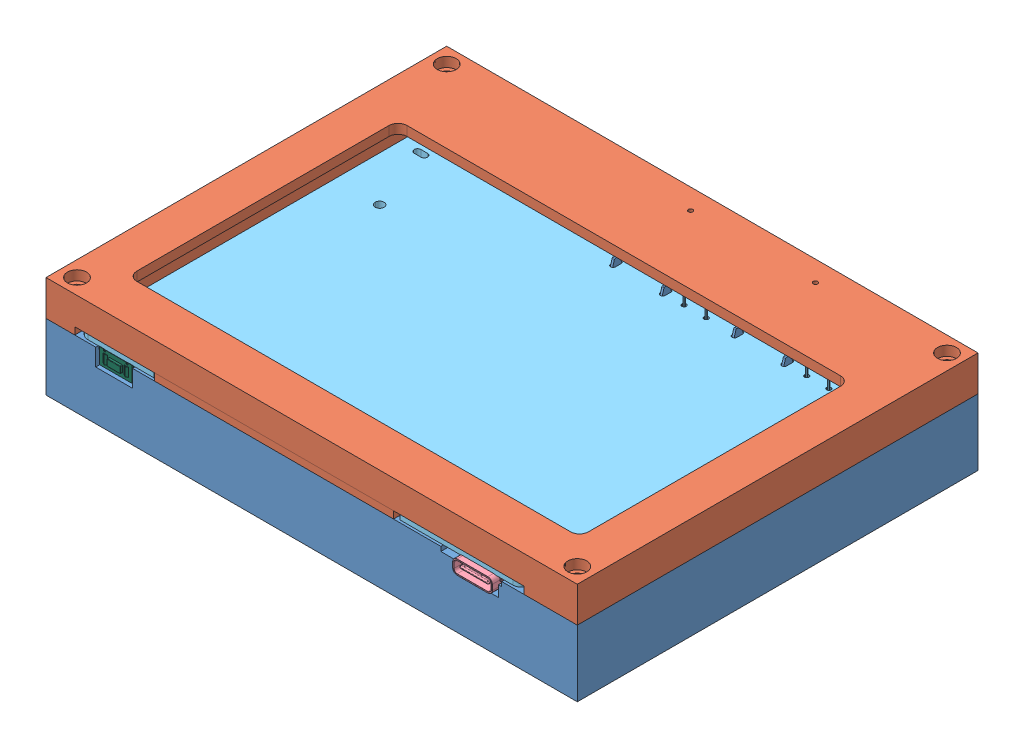
SolidWorks assembly 装配体2, configuration 默认. Lengths in mm.
Overall size (120 23 100.01).
848 component instances, 41 part files, 5 mates.
Components (placement in the parent):
- 底板-1: 底板 [默认] at (-10.6932 -23.0305 0) size (120 15 90.5)
- 面板-1: 面板 [默认] at (-10.6932 -0.0305 0) x (-1 0 0) z (0 0 1) size (120 8 90.5)
- 3D_board_2024-11-06-1: 3D_board_2024-11-06 [默认] at (-63.7814 -6.4105 44.7375) x (1 0 0) z (0 -1 0) size (99.97 100.01 16.2)
  - 3D_board_2024-11-06.step-1: 3D_board_2024-11-06.step [默认] at origin size (99.97 100.01 16.2)
    - iqks-X1.step-1: iqks-X1.step [默认] at (20.955 -9.525 1.5862) x (-1 0 0) z (0 0 1) size (3.2 2.5 0.81)
      - OSC-SMD_4P-L3.2-W2.5-BL.step-1: OSC-SMD_4P-L3.2-W2.5-BL.step [默认] at origin size (3.2 2.5 0.81)
        - SOLID.step-1: SOLID.step [默认] at origin size (3.2 2.5 0.81)
    - iqks-X2.step-1: iqks-X2.step [默认] at (48.2601 -24.765 1.5862) x (-1 0 0) z (0 0 1) size (7 5 1.32)
      - OSC-SMD_4P-L7.0-W5.0-BL.step-1: OSC-SMD_4P-L7.0-W5.0-BL.step [默认] at origin size (7 5 1.32)
        - COMPOUND.step-1: COMPOUND.step [默认] at origin size (7 5 1.32)
    - iqks-U22.step-1: iqks-U22.step [默认] at (45.7201 -54.6101 1.5862) x (-1 0 0) z (0 0 1) size (5.89 7.71 1.66)
      - SSOP-28_L10.2-W5.3-P0.65-LS7.8-BL.step-1: SSOP-28_L10.2-W5.3-P0.65-LS7.8-BL.step [默认] at origin size (5.89 7.71 1.66)
        - SOLID-0.step-1: SOLID-0.step [默认] at origin size (5.89 7.71 1.66)
    - iqks-RN4.step-1: iqks-RN4.step [默认] at (33.0201 -35.5601 1.5862) x (-1 0 0) z (0 0 1) size (3.2 1.6 0.5)
      - RES-ARRAY-SMD_0603-8P-L3.2-W1.6-BL.step-1: RES-ARRAY-SMD_0603-8P-L3.2-W1.6-BL.step [默认] at origin size (3.2 1.6 0.5)
        - COMPOUND-1.step-1: COMPOUND-1.step [默认] at origin size (3.2 1.6 0.5)
    - iqks-RN3.step-1: iqks-RN3.step [默认] at (29.2101 -35.5601 1.5862) x (-1 0 0) z (0 0 1) size (3.2 1.6 0.5)
      - RES-ARRAY-SMD_0603-8P-L3.2-W1.6-BL.step-1: RES-ARRAY-SMD_0603-8P-L3.2-W1.6-BL.step [默认] at origin size (3.2 1.6 0.5)
        - COMPOUND-1.step-1: COMPOUND-1.step [默认] at origin size (3.2 1.6 0.5)
    - iqks-RN2.step-1: iqks-RN2.step [默认] at (25.4001 -35.5601 1.5862) x (-1 0 0) z (0 0 1) size (3.2 1.6 0.5)
      - RES-ARRAY-SMD_0603-8P-L3.2-W1.6-BL.step-1: RES-ARRAY-SMD_0603-8P-L3.2-W1.6-BL.step [默认] at origin size (3.2 1.6 0.5)
        - COMPOUND-1.step-1: COMPOUND-1.step [默认] at origin size (3.2 1.6 0.5)
    - iqks-RN1.step-1: iqks-RN1.step [默认] at (21.59 -35.5601 1.5862) x (-1 0 0) z (0 0 1) size (3.2 1.6 0.5)
      - RES-ARRAY-SMD_0603-8P-L3.2-W1.6-BL.step-1: RES-ARRAY-SMD_0603-8P-L3.2-W1.6-BL.step [默认] at origin size (3.2 1.6 0.5)
        - COMPOUND-1.step-1: COMPOUND-1.step [默认] at origin size (3.2 1.6 0.5)
    - iqks-RN5.step-1: iqks-RN5.step [默认] at (36.8301 -35.5601 1.5862) x (-1 0 0) z (0 0 1) size (3.2 1.6 0.5)
      - RES-ARRAY-SMD_0603-8P-L3.2-W1.6-BL.step-1: RES-ARRAY-SMD_0603-8P-L3.2-W1.6-BL.step [默认] at origin size (3.2 1.6 0.5)
        - COMPOUND-1.step-1: COMPOUND-1.step [默认] at origin size (3.2 1.6 0.5)
    - iqks-R53.step-1: iqks-R53.step [默认] at (90.8052 -10.16 1.5862) x (0 1 0) z (0 0 1) size (1.62 0.81 0.45)
      - R0603.step-1: R0603.step [默认] at origin size (1.62 0.81 0.45)
        - COMPOUND-2.step-1: COMPOUND-2.step [默认] at origin size (1.62 0.81 0.45)
    - iqks-R52.step-1: iqks-R52.step [默认] at (88.9002 -10.16 1.5862) x (0 1 0) z (0 0 1) size (1.62 0.81 0.45)
      - R0603.step-1: R0603.step [默认] at origin size (1.62 0.81 0.45)
        - COMPOUND-2.step-1: COMPOUND-2.step [默认] at origin size (1.62 0.81 0.45)
    - iqks-R7.step-1: iqks-R7.step [默认] at (72.3901 -59.4601 1.5862) size (1.62 0.81 0.45)
      - R0603.step-1: R0603.step [默认] at origin size (1.62 0.81 0.45)
        - COMPOUND-2.step-1: COMPOUND-2.step [默认] at origin size (1.62 0.81 0.45)
    - iqks-R14.step-1: iqks-R14.step [默认] at (82.5502 -59.4601 1.5862) x (-1 0 0) z (0 0 1) size (1.62 0.81 0.45)
      - R0603.step-1: R0603.step [默认] at origin size (1.62 0.81 0.45)
        - COMPOUND-2.step-1: COMPOUND-2.step [默认] at origin size (1.62 0.81 0.45)
    - iqks-R69.step-1: iqks-R69.step [默认] at (50.8001 -40.6401 1.5862) x (0 -1 0) z (0 0 1) size (1.62 0.81 0.45)
      - R0603.step-1: R0603.step [默认] at origin size (1.62 0.81 0.45)
        - COMPOUND-2.step-1: COMPOUND-2.step [默认] at origin size (1.62 0.81 0.45)
    - iqks-R55.step-1: iqks-R55.step [默认] at (84.4552 -10.16 1.5862) x (0 1 0) z (0 0 1) size (1.62 0.81 0.45)
      - R0603.step-1: R0603.step [默认] at origin size (1.62 0.81 0.45)
        - COMPOUND-2.step-1: COMPOUND-2.step [默认] at origin size (1.62 0.81 0.45)
    - iqks-R59.step-1: iqks-R59.step [默认] at (53.3401 -22.86 1.5862) x (0 1 0) z (0 0 1) size (1.62 0.81 0.45)
      - R0603.step-1: R0603.step [默认] at origin size (1.62 0.81 0.45)
        - COMPOUND-2.step-1: COMPOUND-2.step [默认] at origin size (1.62 0.81 0.45)
    - iqks-R62.step-1: iqks-R62.step [默认] at (48.1331 -19.8896 1.5862) x (0.707107 0.707107 0) z (0 0 1) size (1.62 0.81 0.45)
      - R0603.step-1: R0603.step [默认] at origin size (1.62 0.81 0.45)
        - COMPOUND-2.step-1: COMPOUND-2.step [默认] at origin size (1.62 0.81 0.45)
    - iqks-R63.step-1: iqks-R63.step [默认] at (50.8248 -12.6064 1.5862) x (0.707107 -0.707107 0) z (0 0 1) size (1.62 0.81 0.45)
      - R0603.step-1: R0603.step [默认] at origin size (1.62 0.81 0.45)
        - COMPOUND-2.step-1: COMPOUND-2.step [默认] at origin size (1.62 0.81 0.45)
    - iqks-R64.step-1: iqks-R64.step [默认] at (46.3551 -8.255 1.5862) x (-0.707107 0.707107 0) z (0 0 1) size (1.62 0.81 0.45)
      - R0603.step-1: R0603.step [默认] at origin size (1.62 0.81 0.45)
        - COMPOUND-2.step-1: COMPOUND-2.step [默认] at origin size (1.62 0.81 0.45)
    - iqks-R65.step-1: iqks-R65.step [默认] at (10.1012 -43.0318 1.5862) size (1.62 0.81 0.45)
      - R0603.step-1: R0603.step [默认] at origin size (1.62 0.81 0.45)
        - COMPOUND-2.step-1: COMPOUND-2.step [默认] at origin size (1.62 0.81 0.45)
    - iqks-R66.step-1: iqks-R66.step [默认] at (39.3701 -7.62 1.5862) x (0.707107 0.707107 0) z (0 0 1) size (1.62 0.81 0.45)
      - R0603.step-1: R0603.step [默认] at origin size (1.62 0.81 0.45)
        - COMPOUND-2.step-1: COMPOUND-2.step [默认] at origin size (1.62 0.81 0.45)
    - iqks-R67.step-1: iqks-R67.step [默认] at (48.5635 -10.414 1.5862) x (-0.707107 0.707107 0) z (0 0 1) size (1.62 0.81 0.45)
      - R0603.step-1: R0603.step [默认] at origin size (1.62 0.81 0.45)
        - COMPOUND-2.step-1: COMPOUND-2.step [默认] at origin size (1.62 0.81 0.45)
    - iqks-R74.step-1: iqks-R74.step [默认] at (82.5502 -10.16 1.5862) x (0 1 0) z (0 0 1) size (1.62 0.81 0.45)
      - R0603.step-1: R0603.step [默认] at origin size (1.62 0.81 0.45)
        - COMPOUND-2.step-1: COMPOUND-2.step [默认] at origin size (1.62 0.81 0.45)
    - iqks-R75.step-1: iqks-R75.step [默认] at (14.605 -11.303 1.5862) x (0 -1 0) z (0 0 1) size (1.62 0.81 0.45)
      - R0603.step-1: R0603.step [默认] at origin size (1.62 0.81 0.45)
        - COMPOUND-2.step-1: COMPOUND-2.step [默认] at origin size (1.62 0.81 0.45)
    - iqks-R76.step-1: iqks-R76.step [默认] at (33.6551 -8.89 1.5862) size (1.62 0.81 0.45)
      - R0603.step-1: R0603.step [默认] at origin size (1.62 0.81 0.45)
        - COMPOUND-2.step-1: COMPOUND-2.step [默认] at origin size (1.62 0.81 0.45)
    - iqks-R100.step-1: iqks-R100.step [默认] at (43.1801 -47.6251 1.5862) x (0 -1 0) z (0 0 1) size (1.62 0.81 0.45)
      - R0603.step-1: R0603.step [默认] at origin size (1.62 0.81 0.45)
        - COMPOUND-2.step-1: COMPOUND-2.step [默认] at origin size (1.62 0.81 0.45)
    - iqks-R103.step-1: iqks-R103.step [默认] at (54.2291 -36.0681 1.5862) x (-1 0 0) z (0 0 1) size (1.62 0.81 0.45)
      - R0603.step-1: R0603.step [默认] at origin size (1.62 0.81 0.45)
        - COMPOUND-2.step-1: COMPOUND-2.step [默认] at origin size (1.62 0.81 0.45)
    - iqks-R104.step-1: iqks-R104.step [默认] at (54.2291 -37.5921 1.5862) x (-1 0 0) z (0 0 1) size (1.62 0.81 0.45)
      - R0603.step-1: R0603.step [默认] at origin size (1.62 0.81 0.45)
        - COMPOUND-2.step-1: COMPOUND-2.step [默认] at origin size (1.62 0.81 0.45)
    - iqks-R10.step-1: iqks-R10.step [默认] at (79.3752 -65.8101 1.5862) x (0 -1 0) z (0 0 1) size (1.62 0.81 0.45)
      - R0603.step-1: R0603.step [默认] at origin size (1.62 0.81 0.45)
        - COMPOUND-2.step-1: COMPOUND-2.step [默认] at origin size (1.62 0.81 0.45)
    - iqks-R11.step-1: iqks-R11.step [默认] at (75.5652 -65.8101 1.5862) x (0 -1 0) z (0 0 1) size (1.62 0.81 0.45)
      - R0603.step-1: R0603.step [默认] at origin size (1.62 0.81 0.45)
        - COMPOUND-2.step-1: COMPOUND-2.step [默认] at origin size (1.62 0.81 0.45)
    - iqks-R29.step-1: iqks-R29.step [默认] at (93.3452 -65.8101 1.5862) x (0 -1 0) z (0 0 1) size (1.62 0.81 0.45)
      - R0603.step-1: R0603.step [默认] at origin size (1.62 0.81 0.45)
        - COMPOUND-2.step-1: COMPOUND-2.step [默认] at origin size (1.62 0.81 0.45)
    - iqks-R30.step-1: iqks-R30.step [默认] at (89.5352 -65.8101 1.5862) x (0 -1 0) z (0 0 1) size (1.62 0.81 0.45)
      - R0603.step-1: R0603.step [默认] at origin size (1.62 0.81 0.45)
        - COMPOUND-2.step-1: COMPOUND-2.step [默认] at origin size (1.62 0.81 0.45)
    - iqks-R5.step-1: iqks-R5.step [默认] at (87.6302 -65.8101 1.5862) x (0 -1 0) z (0 0 1) size (1.62 0.81 0.45)
      - R0603.step-1: R0603.step [默认] at origin size (1.62 0.81 0.45)
        - COMPOUND-2.step-1: COMPOUND-2.step [默认] at origin size (1.62 0.81 0.45)
    - iqks-R12.step-1: iqks-R12.step [默认] at (81.2802 -65.8101 1.5862) x (0 -1 0) z (0 0 1) size (1.62 0.81 0.45)
      - R0603.step-1: R0603.step [默认] at origin size (1.62 0.81 0.45)
        - COMPOUND-2.step-1: COMPOUND-2.step [默认] at origin size (1.62 0.81 0.45)
    - iqks-R13.step-1: iqks-R13.step [默认] at (73.6601 -65.8101 1.5862) x (0 -1 0) z (0 0 1) size (1.62 0.81 0.45)
      - R0603.step-1: R0603.step [默认] at origin size (1.62 0.81 0.45)
        - COMPOUND-2.step-1: COMPOUND-2.step [默认] at origin size (1.62 0.81 0.45)
    - iqks-R31.step-1: iqks-R31.step [默认] at (95.2502 -65.8101 1.5862) x (0 -1 0) z (0 0 1) size (1.62 0.81 0.45)
      - R0603.step-1: R0603.step [默认] at origin size (1.62 0.81 0.45)
        - COMPOUND-2.step-1: COMPOUND-2.step [默认] at origin size (1.62 0.81 0.45)
    - iqks-R115.step-1: iqks-R115.step [默认] at (83.8202 -29.8451 1.5862) x (-1 0 0) z (0 0 1) size (1.62 0.81 0.45)
      - R0603.step-1: R0603.step [默认] at origin size (1.62 0.81 0.45)
        - COMPOUND-2.step-1: COMPOUND-2.step [默认] at origin size (1.62 0.81 0.45)
    - iqks-R122.step-1: iqks-R122.step [默认] at (76.8352 -41.0211 1.5862) x (-1 0 0) z (0 0 1) size (1.62 0.81 0.45)
      - R0603.step-1: R0603.step [默认] at origin size (1.62 0.81 0.45)
        - COMPOUND-2.step-1: COMPOUND-2.step [默认] at origin size (1.62 0.81 0.45)
    - iqks-R91.step-1: iqks-R91.step [默认] at (42.5451 -61.5951 1.5862) x (0 -1 0) z (0 0 1) size (1.62 0.81 0.45)
      - R0603.step-1: R0603.step [默认] at origin size (1.62 0.81 0.45)
        - COMPOUND-2.step-1: COMPOUND-2.step [默认] at origin size (1.62 0.81 0.45)
    - iqks-R92.step-1: iqks-R92.step [默认] at (48.8951 -47.6251 1.5862) x (0 -1 0) z (0 0 1) size (1.62 0.81 0.45)
      - R0603.step-1: R0603.step [默认] at origin size (1.62 0.81 0.45)
        - COMPOUND-2.step-1: COMPOUND-2.step [默认] at origin size (1.62 0.81 0.45)
    - iqks-R111.step-1: iqks-R111.step [默认] at (24.765 -60.9601 1.5862) x (0 1 0) z (0 0 1) size (1.62 0.81 0.45)
      - R0603.step-1: R0603.step [默认] at origin size (1.62 0.81 0.45)
        - COMPOUND-2.step-1: COMPOUND-2.step [默认] at origin size (1.62 0.81 0.45)
    - iqks-R112.step-1: iqks-R112.step [默认] at (86.3602 -27.3051 1.5862) x (0 -1 0) z (0 0 1) size (1.62 0.81 0.45)
      - R0603.step-1: R0603.step [默认] at origin size (1.62 0.81 0.45)
        - COMPOUND-2.step-1: COMPOUND-2.step [默认] at origin size (1.62 0.81 0.45)
    - iqks-R128.step-1: iqks-R128.step [默认] at (73.1521 -51.8161 1.5862) x (0 -1 0) z (0 0 1) size (1.62 0.81 0.45)
      - R0603.step-1: R0603.step [默认] at origin size (1.62 0.81 0.45)
        - COMPOUND-2.step-1: COMPOUND-2.step [默认] at origin size (1.62 0.81 0.45)
    - iqks-R113.step-1: iqks-R113.step [默认] at (77.4702 -24.765 1.5862) x (0 1 0) z (0 0 1) size (1.62 0.81 0.45)
      - R0603.step-1: R0603.step [默认] at origin size (1.62 0.81 0.45)
        - COMPOUND-2.step-1: COMPOUND-2.step [默认] at origin size (1.62 0.81 0.45)
    - iqks-R6.step-1: iqks-R6.step [默认] at (86.3602 -59.4601 1.5862) size (1.62 0.81 0.45)
      - R0603.step-1: R0603.step [默认] at origin size (1.62 0.81 0.45)
        - COMPOUND-2.step-1: COMPOUND-2.step [默认] at origin size (1.62 0.81 0.45)
    - iqks-R32.step-1: iqks-R32.step [默认] at (96.5202 -59.4601 1.5862) x (-1 0 0) z (0 0 1) size (1.62 0.81 0.45)
      - R0603.step-1: R0603.step [默认] at origin size (1.62 0.81 0.45)
        - COMPOUND-2.step-1: COMPOUND-2.step [默认] at origin size (1.62 0.81 0.45)
    - iqks-R9.step-1: iqks-R9.step [默认] at (91.4402 -65.8101 1.5862) x (0 1 0) z (0 0 1) size (1.62 0.81 0.45)
      - R0603.step-1: R0603.step [默认] at origin size (1.62 0.81 0.45)
        - COMPOUND-2.step-1: COMPOUND-2.step [默认] at origin size (1.62 0.81 0.45)
    - iqks-R16.step-1: iqks-R16.step [默认] at (77.4702 -65.8101 1.5862) x (0 1 0) z (0 0 1) size (1.62 0.81 0.45)
      - R0603.step-1: R0603.step [默认] at origin size (1.62 0.81 0.45)
        - COMPOUND-2.step-1: COMPOUND-2.step [默认] at origin size (1.62 0.81 0.45)
    - iqks-R48.step-1: iqks-R48.step [默认] at (86.9952 -10.16 1.5862) x (0 1 0) z (0 0 1) size (1.62 0.81 0.45)
      - R0603.step-1: R0603.step [默认] at origin size (1.62 0.81 0.45)
        - COMPOUND-2.step-1: COMPOUND-2.step [默认] at origin size (1.62 0.81 0.45)
    - iqks-R50.step-1: iqks-R50.step [默认] at (92.7102 -10.16 1.5862) x (0 1 0) z (0 0 1) size (1.62 0.81 0.45)
      - R0603.step-1: R0603.step [默认] at origin size (1.62 0.81 0.45)
        - COMPOUND-2.step-1: COMPOUND-2.step [默认] at origin size (1.62 0.81 0.45)
    - iqks-R114.step-1: iqks-R114.step [默认] at (80.6452 -29.8451 1.5862) x (-1 0 0) z (0 0 1) size (1.62 0.81 0.45)
      - R0603.step-1: R0603.step [默认] at origin size (1.62 0.81 0.45)
        - COMPOUND-2.step-1: COMPOUND-2.step [默认] at origin size (1.62 0.81 0.45)
    - iqks-R21.step-1: iqks-R21.step [默认] at (19.685 -71.1201 1.5862) x (0 -1 0) z (0 0 1) size (1.62 0.81 0.45)
      - R0603.step-1: R0603.step [默认] at origin size (1.62 0.81 0.45)
        - COMPOUND-2.step-1: COMPOUND-2.step [默认] at origin size (1.62 0.81 0.45)
    - iqks-R22.step-1: iqks-R22.step [默认] at (19.685 -74.9301 1.5862) x (0 -1 0) z (0 0 1) size (1.62 0.81 0.45)
      - R0603.step-1: R0603.step [默认] at origin size (1.62 0.81 0.45)
        - COMPOUND-2.step-1: COMPOUND-2.step [默认] at origin size (1.62 0.81 0.45)
    - iqks-R25.step-1: iqks-R25.step [默认] at (34.2901 -71.1201 1.5862) x (0 -1 0) z (0 0 1) size (1.62 0.81 0.45)
      - R0603.step-1: R0603.step [默认] at origin size (1.62 0.81 0.45)
        - COMPOUND-2.step-1: COMPOUND-2.step [默认] at origin size (1.62 0.81 0.45)
    - iqks-R26.step-1: iqks-R26.step [默认] at (34.2901 -74.9301 1.5862) x (0 -1 0) z (0 0 1) size (1.62 0.81 0.45)
      - R0603.step-1: R0603.step [默认] at origin size (1.62 0.81 0.45)
        - COMPOUND-2.step-1: COMPOUND-2.step [默认] at origin size (1.62 0.81 0.45)
    - iqks-R116.step-1: iqks-R116.step [默认] at (96.5202 -26.6701 1.5862) x (0 1 0) z (0 0 1) size (1.62 0.81 0.45)
      - R0603.step-1: R0603.step [默认] at origin size (1.62 0.81 0.45)
        - COMPOUND-2.step-1: COMPOUND-2.step [默认] at origin size (1.62 0.81 0.45)
    - iqks-R2.step-1: iqks-R2.step [默认] at (21.59 -71.1201 1.5862) x (0 -1 0) z (0 0 1) size (1.62 0.81 0.45)
      - R0603.step-1: R0603.step [默认] at origin size (1.62 0.81 0.45)
        - COMPOUND-2.step-1: COMPOUND-2.step [默认] at origin size (1.62 0.81 0.45)
    - iqks-R4.step-1: iqks-R4.step [默认] at (21.59 -74.9301 1.5862) x (0 1 0) z (0 0 1) size (1.62 0.81 0.45)
      - R0603.step-1: R0603.step [默认] at origin size (1.62 0.81 0.45)
        - COMPOUND-2.step-1: COMPOUND-2.step [默认] at origin size (1.62 0.81 0.45)
    - iqks-R19.step-1: iqks-R19.step [默认] at (36.1951 -71.1201 1.5862) x (0 -1 0) z (0 0 1) size (1.62 0.81 0.45)
      - R0603.step-1: R0603.step [默认] at origin size (1.62 0.81 0.45)
        - COMPOUND-2.step-1: COMPOUND-2.step [默认] at origin size (1.62 0.81 0.45)
    - iqks-R20.step-1: iqks-R20.step [默认] at (36.1951 -74.9301 1.5862) x (0 1 0) z (0 0 1) size (1.62 0.81 0.45)
      - R0603.step-1: R0603.step [默认] at origin size (1.62 0.81 0.45)
        - COMPOUND-2.step-1: COMPOUND-2.step [默认] at origin size (1.62 0.81 0.45)
    - iqks-R110.step-1: iqks-R110.step [默认] at (22.86 -60.9601 1.5862) x (0 1 0) z (0 0 1) size (1.62 0.81 0.45)
      - R0603.step-1: R0603.step [默认] at origin size (1.62 0.81 0.45)
        - COMPOUND-2.step-1: COMPOUND-2.step [默认] at origin size (1.62 0.81 0.45)
    - iqks-R117.step-1: iqks-R117.step [默认] at (93.9802 -26.0351 1.5862) x (-1 0 0) z (0 0 1) size (1.62 0.81 0.45)
      - R0603.step-1: R0603.step [默认] at origin size (1.62 0.81 0.45)
        - COMPOUND-2.step-1: COMPOUND-2.step [默认] at origin size (1.62 0.81 0.45)
    - iqks-R1.step-1: iqks-R1.step [默认] at (10.16 -67.3101 1.5862) x (0 -1 0) z (0 0 1) size (1.62 0.81 0.45)
      - R0603.step-1: R0603.step [默认] at origin size (1.62 0.81 0.45)
        - COMPOUND-2.step-1: COMPOUND-2.step [默认] at origin size (1.62 0.81 0.45)
    - iqks-R3.step-1: iqks-R3.step [默认] at (22.86 -67.3101 1.5862) x (0 -1 0) z (0 0 1) size (1.62 0.81 0.45)
      - R0603.step-1: R0603.step [默认] at origin size (1.62 0.81 0.45)
        - COMPOUND-2.step-1: COMPOUND-2.step [默认] at origin size (1.62 0.81 0.45)
    - iqks-R17.step-1: iqks-R17.step [默认] at (37.4651 -67.3101 1.5862) x (0 -1 0) z (0 0 1) size (1.62 0.81 0.45)
      - R0603.step-1: R0603.step [默认] at origin size (1.62 0.81 0.45)
        - COMPOUND-2.step-1: COMPOUND-2.step [默认] at origin size (1.62 0.81 0.45)
    - iqks-R18.step-1: iqks-R18.step [默认] at (24.765 -67.3101 1.5862) x (0 -1 0) z (0 0 1) size (1.62 0.81 0.45)
      - R0603.step-1: R0603.step [默认] at origin size (1.62 0.81 0.45)
        - COMPOUND-2.step-1: COMPOUND-2.step [默认] at origin size (1.62 0.81 0.45)
    - iqks-R121.step-1: iqks-R121.step [默认] at (86.8682 -20.32 1.5862) x (0 1 0) z (0 0 1) size (1.62 0.81 0.45)
      - R0603.step-1: R0603.step [默认] at origin size (1.62 0.81 0.45)
        - COMPOUND-2.step-1: COMPOUND-2.step [默认] at origin size (1.62 0.81 0.45)
    - iqks-R120.step-1: iqks-R120.step [默认] at (86.1062 -17.78 1.5862) x (-1 0 0) z (0 0 1) size (1.62 0.81 0.45)
      - R0603.step-1: R0603.step [默认] at origin size (1.62 0.81 0.45)
        - COMPOUND-2.step-1: COMPOUND-2.step [默认] at origin size (1.62 0.81 0.45)
    - iqks-R118.step-1: iqks-R118.step [默认] at (80.8992 -4.699 1.5862) x (-1 0 0) z (0 0 1) size (1.62 0.81 0.45)
      - R0603.step-1: R0603.step [默认] at origin size (1.62 0.81 0.45)
        - COMPOUND-2.step-1: COMPOUND-2.step [默认] at origin size (1.62 0.81 0.45)
    - iqks-R119.step-1: iqks-R119.step [默认] at (83.5662 -17.145 1.5862) x (0 -1 0) z (0 0 1) size (1.62 0.81 0.45)
      - R0603.step-1: R0603.step [默认] at origin size (1.62 0.81 0.45)
        - COMPOUND-2.step-1: COMPOUND-2.step [默认] at origin size (1.62 0.81 0.45)
    - iqks-R23.step-1: iqks-R23.step [默认] at (15.24 -75.5652 1.5862) x (-1 0 0) z (0 0 1) size (1.62 0.81 0.45)
      - R0603.step-1: R0603.step [默认] at origin size (1.62 0.81 0.45)
        - COMPOUND-2.step-1: COMPOUND-2.step [默认] at origin size (1.62 0.81 0.45)
    - iqks-R24.step-1: iqks-R24.step [默认] at (12.065 -75.5652 1.5862) x (-1 0 0) z (0 0 1) size (1.62 0.81 0.45)
      - R0603.step-1: R0603.step [默认] at origin size (1.62 0.81 0.45)
        - COMPOUND-2.step-1: COMPOUND-2.step [默认] at origin size (1.62 0.81 0.45)
    - iqks-R27.step-1: iqks-R27.step [默认] at (29.8451 -75.5652 1.5862) x (-1 0 0) z (0 0 1) size (1.62 0.81 0.45)
      - R0603.step-1: R0603.step [默认] at origin size (1.62 0.81 0.45)
        - COMPOUND-2.step-1: COMPOUND-2.step [默认] at origin size (1.62 0.81 0.45)
    - iqks-R28.step-1: iqks-R28.step [默认] at (26.6701 -75.5652 1.5862) x (-1 0 0) z (0 0 1) size (1.62 0.81 0.45)
      - R0603.step-1: R0603.step [默认] at origin size (1.62 0.81 0.45)
        - COMPOUND-2.step-1: COMPOUND-2.step [默认] at origin size (1.62 0.81 0.45)
    - iqks-R123.step-1: iqks-R123.step [默认] at (74.9301 -51.8161 1.5862) x (0 -1 0) z (0 0 1) size (1.62 0.81 0.45)
      - R0603.step-1: R0603.step [默认] at origin size (1.62 0.81 0.45)
        - COMPOUND-2.step-1: COMPOUND-2.step [默认] at origin size (1.62 0.81 0.45)
    - iqks-R49.step-1: iqks-R49.step [默认] at (95.2502 -10.16 1.5862) x (0 1 0) z (0 0 1) size (1.62 0.81 0.45)
      - R0603.step-1: R0603.step [默认] at origin size (1.62 0.81 0.45)
        - COMPOUND-2.step-1: COMPOUND-2.step [默认] at origin size (1.62 0.81 0.45)
    - iqks-R124.step-1: iqks-R124.step [默认] at (84.4552 -46.1011 1.5862) x (0 1 0) z (0 0 1) size (1.62 0.81 0.45)
      - R0603.step-1: R0603.step [默认] at origin size (1.62 0.81 0.45)
        - COMPOUND-2.step-1: COMPOUND-2.step [默认] at origin size (1.62 0.81 0.45)
    - iqks-R125.step-1: iqks-R125.step [默认] at (88.2652 -46.1011 1.5862) x (0 1 0) z (0 0 1) size (1.62 0.81 0.45)
      - R0603.step-1: R0603.step [默认] at origin size (1.62 0.81 0.45)
        - COMPOUND-2.step-1: COMPOUND-2.step [默认] at origin size (1.62 0.81 0.45)
    - iqks-R126.step-1: iqks-R126.step [默认] at (80.6452 -51.8161 1.5862) x (0 -1 0) z (0 0 1) size (1.62 0.81 0.45)
      - R0603.step-1: R0603.step [默认] at origin size (1.62 0.81 0.45)
        - COMPOUND-2.step-1: COMPOUND-2.step [默认] at origin size (1.62 0.81 0.45)
    - iqks-R127.step-1: iqks-R127.step [默认] at (78.7402 -51.8161 1.5862) x (0 1 0) z (0 0 1) size (1.62 0.81 0.45)
      - R0603.step-1: R0603.step [默认] at origin size (1.62 0.81 0.45)
        - COMPOUND-2.step-1: COMPOUND-2.step [默认] at origin size (1.62 0.81 0.45)
    - iqks-R129.step-1: iqks-R129.step [默认] at (68.9593 -45.3937 1.5862) x (0 -1 0) z (0 0 1) size (1.62 0.81 0.45)
      - R0603.step-1: R0603.step [默认] at origin size (1.62 0.81 0.45)
        - COMPOUND-2.step-1: COMPOUND-2.step [默认] at origin size (1.62 0.81 0.45)
    - iqks-R131.step-1: iqks-R131.step [默认] at (97.4092 -49.5301 1.5862) x (0 -1 0) z (0 0 1) size (1.62 0.81 0.45)
      - R0603.step-1: R0603.step [默认] at origin size (1.62 0.81 0.45)
        - COMPOUND-2.step-1: COMPOUND-2.step [默认] at origin size (1.62 0.81 0.45)
    - iqks-R132.step-1: iqks-R132.step [默认] at (94.8692 -50.8001 1.5862) x (-1 0 0) z (0 0 1) size (1.62 0.81 0.45)
      - R0603.step-1: R0603.step [默认] at origin size (1.62 0.81 0.45)
        - COMPOUND-2.step-1: COMPOUND-2.step [默认] at origin size (1.62 0.81 0.45)
    - iqks-R133.step-1: iqks-R133.step [默认] at (66.4193 -46.1557 1.5862) x (-1 0 0) z (0 0 1) size (1.62 0.81 0.45)
      - R0603.step-1: R0603.step [默认] at origin size (1.62 0.81 0.45)
        - COMPOUND-2.step-1: COMPOUND-2.step [默认] at origin size (1.62 0.81 0.45)
    - iqks-JP1.step-1: iqks-JP1.step [默认] at (93.9802 -29.8451 1.5862) x (-1 0 0) z (0 0 1) size (1.62 0.81 0.45)
      - R0603.step-1: R0603.step [默认] at origin size (1.62 0.81 0.45)
        - COMPOUND-2.step-1: COMPOUND-2.step [默认] at origin size (1.62 0.81 0.45)
    - iqks-JP2.step-1: iqks-JP2.step [默认] at (86.1062 -15.875 1.5862) x (-1 0 0) z (0 0 1) size (1.62 0.81 0.45)
      - R0603.step-1: R0603.step [默认] at origin size (1.62 0.81 0.45)
        - COMPOUND-2.step-1: COMPOUND-2.step [默认] at origin size (1.62 0.81 0.45)
    - iqks-JP4.step-1: iqks-JP4.step [默认] at (33.6551 -6.985 1.5862) size (1.62 0.81 0.45)
      - R0603.step-1: R0603.step [默认] at origin size (1.62 0.81 0.45)
        - COMPOUND-2.step-1: COMPOUND-2.step [默认] at origin size (1.62 0.81 0.45)
    - iqks-JP5.step-1: iqks-JP5.step [默认] at (92.0752 -49.7841 1.5862) x (0 -1 0) z (0 0 1) size (1.62 0.81 0.45)
      - R0603.step-1: R0603.step [默认] at origin size (1.62 0.81 0.45)
        - COMPOUND-2.step-1: COMPOUND-2.step [默认] at origin size (1.62 0.81 0.45)
    - iqks-JP6.step-1: iqks-JP6.step [默认] at (62.5179 -40.2999 1.5862) x (0 -1 0) z (0 0 1) size (1.62 0.81 0.45)
      - R0603.step-1: R0603.step [默认] at origin size (1.62 0.81 0.45)
        - COMPOUND-2.step-1: COMPOUND-2.step [默认] at origin size (1.62 0.81 0.45)
    - iqks-R101.step-1: iqks-R101.step [默认] at (64.1351 -50.8001 1.5862) x (0 1 0) z (0 0 1) size (1.62 0.81 0.45)
      - R0603.step-1: R0603.step [默认] at origin size (1.62 0.81 0.45)
        - COMPOUND-2.step-1: COMPOUND-2.step [默认] at origin size (1.62 0.81 0.45)
    - iqks-R102.step-1: iqks-R102.step [默认] at (66.0401 -50.8001 1.5862) x (0 1 0) z (0 0 1) size (1.62 0.81 0.45)
      - R0603.step-1: R0603.step [默认] at origin size (1.62 0.81 0.45)
        - COMPOUND-2.step-1: COMPOUND-2.step [默认] at origin size (1.62 0.81 0.45)
    - iqks-R109.step-1: iqks-R109.step [默认] at (43.1801 -26.0351 1.5862) x (0 1 0) z (0 0 1) size (1.62 0.81 0.45)
      - R0603.step-1: R0603.step [默认] at origin size (1.62 0.81 0.45)
        - COMPOUND-2.step-1: COMPOUND-2.step [默认] at origin size (1.62 0.81 0.45)
    - iqks-R134.step-1: iqks-R134.step [默认] at (80.0102 -77.9782 0) x (0 -1 0) z (0 0 -1) size (1.62 0.81 0.45)
      - R0603.step-1: R0603.step [默认] at origin size (1.62 0.81 0.45)
        - COMPOUND-2.step-1: COMPOUND-2.step [默认] at origin size (1.62 0.81 0.45)
    - iqks-R135.step-1: iqks-R135.step [默认] at (51.5621 -77.8512 0) x (0 -1 0) z (0 0 -1) size (1.62 0.81 0.45)
      - R0603.step-1: R0603.step [默认] at origin size (1.62 0.81 0.45)
        - COMPOUND-2.step-1: COMPOUND-2.step [默认] at origin size (1.62 0.81 0.45)
    - iqks-R138.step-1: iqks-R138.step [默认] at (9.779 -8.636 1.5862) x (-1 0 0) z (0 0 1) size (1.62 0.81 0.45)
      - R0603.step-1: R0603.step [默认] at origin size (1.62 0.81 0.45)
        - COMPOUND-2.step-1: COMPOUND-2.step [默认] at origin size (1.62 0.81 0.45)
    - iqks-R139.step-1: iqks-R139.step [默认] at (9.779 -10.414 1.5862) size (1.62 0.81 0.45)
      - R0603.step-1: R0603.step [默认] at origin size (1.62 0.81 0.45)
        - COMPOUND-2.step-1: COMPOUND-2.step [默认] at origin size (1.62 0.81 0.45)
    - iqks-R8.step-1: iqks-R8.step [默认] at (71.3741 -82.0822 1.5862) x (-1 0 0) z (0 0 1) size (1.62 0.81 0.45)
      - R0603.step-1: R0603.step [默认] at origin size (1.62 0.81 0.45)
        - COMPOUND-2.step-1: COMPOUND-2.step [默认] at origin size (1.62 0.81 0.45)
    - iqks-R15.step-1: iqks-R15.step [默认] at (64.0081 -82.0822 1.5862) size (1.62 0.81 0.45)
      - R0603.step-1: R0603.step [默认] at origin size (1.62 0.81 0.45)
        - COMPOUND-2.step-1: COMPOUND-2.step [默认] at origin size (1.62 0.81 0.45)
    - iqks-J8.step-1: iqks-J8.step [默认] at (4.826 -52.5781 1.5862) x (0 1 0) z (0 0 1) size (1.62 0.81 0.45)
      - R0603.step-1: R0603.step [默认] at origin size (1.62 0.81 0.45)
        - COMPOUND-2.step-1: COMPOUND-2.step [默认] at origin size (1.62 0.81 0.45)
    - iqks-J9.step-1: iqks-J9.step [默认] at (91.5672 -68.8341 1.5862) x (-1 0 0) z (0 0 1) size (1.62 0.81 0.45)
      - R0603.step-1: R0603.step [默认] at origin size (1.62 0.81 0.45)
        - COMPOUND-2.step-1: COMPOUND-2.step [默认] at origin size (1.62 0.81 0.45)
    - iqks-J10.step-1: iqks-J10.step [默认] at (69.3143 -63.9872 1.5862) x (0 -1 0) z (0 0 1) size (1.62 0.81 0.45)
      - R0603.step-1: R0603.step [默认] at origin size (1.62 0.81 0.45)
        - COMPOUND-2.step-1: COMPOUND-2.step [默认] at origin size (1.62 0.81 0.45)
    - iqks-R60.step-1: iqks-R60.step [默认] at (13.2762 -43.0318 1.5862) size (1.62 0.81 0.45)
      - R0603.step-1: R0603.step [默认] at origin size (1.62 0.81 0.45)
        - COMPOUND-2.step-1: COMPOUND-2.step [默认] at origin size (1.62 0.81 0.45)
    - iqks-SW3.step-1: iqks-SW3.step [默认] at (6.604 -14.986 1.5862) size (8 3.3 5)
      - SW-SMD_L6.0-W3.3-LS8.0.step-1: SW-SMD_L6.0-W3.3-LS8.0.step [默认] at origin size (8 3.3 5)
        - SOLID-3.step-1: SOLID-3.step [默认] at origin size (8 3.3 5)
    - iqks-C130.step-1: iqks-C130.step [默认] at (94.6152 -56.9201 1.5862) size (3.2 2.52 0.9)
      - C1210.step-1: C1210.step [默认] at origin size (3.2 2.52 0.9)
        - SOLID-4.step-1: SOLID-4.step [默认] at origin size (3.2 2.52 0.9)
    - iqks-C35.step-1: iqks-C35.step [默认] at (88.2652 -56.9201 1.5862) x (-1 0 0) z (0 0 1) size (3.2 2.52 0.9)
      - C1210.step-1: C1210.step [默认] at origin size (3.2 2.52 0.9)
        - SOLID-4.step-1: SOLID-4.step [默认] at origin size (3.2 2.52 0.9)
    - iqks-C34.step-1: iqks-C34.step [默认] at (80.6452 -56.9201 1.5862) size (3.2 2.52 0.9)
      - C1210.step-1: C1210.step [默认] at origin size (3.2 2.52 0.9)
        - SOLID-4.step-1: SOLID-4.step [默认] at origin size (3.2 2.52 0.9)
    - iqks-C131.step-1: iqks-C131.step [默认] at (74.2951 -56.9201 1.5862) x (-1 0 0) z (0 0 1) size (3.2 2.52 0.9)
      - C1210.step-1: C1210.step [默认] at origin size (3.2 2.52 0.9)
        - SOLID-4.step-1: SOLID-4.step [默认] at origin size (3.2 2.52 0.9)
    - iqks-D7.step-1: iqks-D7.step [默认] at (3.81 -62.8651 1.5862) size (2.5 1.3 1.1)
      - SOD-323_L1.7-W1.3-LS2.5-BI.step-1: SOD-323_L1.7-W1.3-LS2.5-BI.step [默认] at origin size (2.5 1.3 1.1)
        - COMPOUND-5.step-1: COMPOUND-5.step [默认] at origin size (2.5 1.3 1.1)
    - iqks-D6.step-1: iqks-D6.step [默认] at (3.81 -58.4201 1.5862) x (-1 0 0) z (0 0 1) size (2.5 1.3 1.1)
      - SOD-323_L1.7-W1.3-LS2.5-BI.step-1: SOD-323_L1.7-W1.3-LS2.5-BI.step [默认] at origin size (2.5 1.3 1.1)
        - COMPOUND-5.step-1: COMPOUND-5.step [默认] at origin size (2.5 1.3 1.1)
    - iqks-D8.step-1: iqks-D8.step [默认] at (97.6632 -15.113 1.5862) x (0 -1 0) z (0 0 1) size (2.5 1.3 1.1)
      - SOD-323_L1.7-W1.3-LS2.5-BI.step-1: SOD-323_L1.7-W1.3-LS2.5-BI.step [默认] at origin size (2.5 1.3 1.1)
        - COMPOUND-5.step-1: COMPOUND-5.step [默认] at origin size (2.5 1.3 1.1)
    - iqks-D5.step-1: iqks-D5.step [默认] at (3.81 -67.3101 1.5862) size (2.5 1.3 1.1)
      - SOD-323_L1.7-W1.3-LS2.5-BI.step-1: SOD-323_L1.7-W1.3-LS2.5-BI.step [默认] at origin size (2.5 1.3 1.1)
        - COMPOUND-5.step-1: COMPOUND-5.step [默认] at origin size (2.5 1.3 1.1)
    - iqks-D4.step-1: iqks-D4.step [默认] at (13.9112 -49.3818 1.5862) x (0 -1 0) z (0 0 1) size (3.68 1.6 1.22)
      - SOD-123_L2.8-W1.8-LS3.7-RD.step-1: SOD-123_L2.8-W1.8-LS3.7-RD.step [默认] at origin size (3.68 1.6 1.22)
        - SOLID-6.step-1: SOLID-6.step [默认] at origin size (3.68 1.6 1.22)
    - iqks-L2.step-1: iqks-L2.step [默认] at (85.0902 -38.4811 1.5862) x (0 1 0) z (0 0 1) size (4.4 4.2 2.1)
      - IND-SMD_L4.4-W4.2.step-1: IND-SMD_L4.4-W4.2.step [默认] at origin size (4.4 4.2 2.1)
        - SOLID-7.step-1: SOLID-7.step [默认] at origin size (4.4 4.2 2.1)
    - iqks-L3.step-1: iqks-L3.step [默认] at (72.3901 -46.7361 1.5862) x (0 1 0) z (0 0 1) size (4.4 4.2 2.1)
      - IND-SMD_L4.4-W4.2.step-1: IND-SMD_L4.4-W4.2.step [默认] at origin size (4.4 4.2 2.1)
        - SOLID-7.step-1: SOLID-7.step [默认] at origin size (4.4 4.2 2.1)
    - iqks-L7.step-1: iqks-L7.step [默认] at (10.1012 -50.0168 1.5862) size (4.4 4.2 2.1)
      - IND-SMD_L4.4-W4.2.step-1: IND-SMD_L4.4-W4.2.step [默认] at origin size (4.4 4.2 2.1)
        - SOLID-7.step-1: SOLID-7.step [默认] at origin size (4.4 4.2 2.1)
    - iqks-U20.step-1: iqks-U20.step [默认] at (10.795 -28.5751 1.5862) size (5.3 7.91 2.07)
      - SOIC-8_L5.3-W5.3-P1.27-LS8.0-BL.step-1: SOIC-8_L5.3-W5.3-P1.27-LS8.0-BL.step [默认] at origin size (5.3 7.91 2.07)
        - COMPOUND-8.step-1: COMPOUND-8.step [默认] at origin size (5.3 7.91 2.07)
    - iqks-C40.step-1: iqks-C40.step [默认] at (94.3612 -72.5251 1.5862) size (7.2 5 13.3)
      - CAP-TH_L7.2-W5.0-P5.00-D1.0.step-1: CAP-TH_L7.2-W5.0-P5.00-D1.0.step [默认] at origin size (7.2 5 13.3)
        - SOLID-9.step-1: SOLID-9.step [默认] at origin size (7.2 5 13.3)
    - iqks-C12.step-1: iqks-C12.step [默认] at (66.6751 -78.2402 1.5862) size (7.2 5 13.3)
      - CAP-TH_L7.2-W5.0-P5.00-D1.0.step-1: CAP-TH_L7.2-W5.0-P5.00-D1.0.step [默认] at origin size (7.2 5 13.3)
        - SOLID-9.step-1: SOLID-9.step [默认] at origin size (7.2 5 13.3)
    - iqks-C47.step-1: iqks-C47.step [默认] at (66.6751 -72.5251 1.5862) size (7.2 5 13.3)
      - CAP-TH_L7.2-W5.0-P5.00-D1.0.step-1: CAP-TH_L7.2-W5.0-P5.00-D1.0.step [默认] at origin size (7.2 5 13.3)
        - SOLID-9.step-1: SOLID-9.step [默认] at origin size (7.2 5 13.3)
    - iqks-C41.step-1: iqks-C41.step [默认] at (94.3612 -78.2402 1.5862) size (7.2 5 13.3)
      - CAP-TH_L7.2-W5.0-P5.00-D1.0.step-1: CAP-TH_L7.2-W5.0-P5.00-D1.0.step [默认] at origin size (7.2 5 13.3)
        - SOLID-9.step-1: SOLID-9.step [默认] at origin size (7.2 5 13.3)
    - iqks-C114.step-1: iqks-C114.step [默认] at (45.0851 -47.6251 1.5862) x (0 1 0) z (0 0 1) size (1.6 0.8 0.8)
      - C0603.step-1: C0603.step [默认] at origin size (1.6 0.8 0.8)
        - SOLID-10.step-1: SOLID-10.step [默认] at origin size (1.6 0.8 0.8)
    - iqks-C102.step-1: iqks-C102.step [默认] at (17.78 -21.844 1.5862) x (-1 0 0) z (0 0 1) size (1.6 0.8 0.8)
      - C0603.step-1: C0603.step [默认] at origin size (1.6 0.8 0.8)
        - SOLID-10.step-1: SOLID-10.step [默认] at origin size (1.6 0.8 0.8)
    - iqks-C101.step-1: iqks-C101.step [默认] at (8.5117 -21.8363 1.5862) x (0 1 0) z (0 0 1) size (1.6 0.8 0.8)
      - C0603.step-1: C0603.step [默认] at origin size (1.6 0.8 0.8)
        - SOLID-10.step-1: SOLID-10.step [默认] at origin size (1.6 0.8 0.8)
    - iqks-C100.step-1: iqks-C100.step [默认] at (21.59 -45.5931 1.5862) x (-1 0 0) z (0 0 1) size (1.6 0.8 0.8)
      - C0603.step-1: C0603.step [默认] at origin size (1.6 0.8 0.8)
        - SOLID-10.step-1: SOLID-10.step [默认] at origin size (1.6 0.8 0.8)
    - iqks-C93.step-1: iqks-C93.step [默认] at (13.9112 -45.5718 1.5862) x (0 1 0) z (0 0 1) size (1.6 0.8 0.8)
      - C0603.step-1: C0603.step [默认] at origin size (1.6 0.8 0.8)
        - SOLID-10.step-1: SOLID-10.step [默认] at origin size (1.6 0.8 0.8)
    - iqks-C92.step-1: iqks-C92.step [默认] at (50.8001 -36.765 1.5862) x (0 1 0) z (0 0 1) size (1.6 0.8 0.8)
      - C0603.step-1: C0603.step [默认] at origin size (1.6 0.8 0.8)
        - SOLID-10.step-1: SOLID-10.step [默认] at origin size (1.6 0.8 0.8)
    - iqks-C91.step-1: iqks-C91.step [默认] at (36.9571 -10.033 1.5862) x (-0.707107 -0.707107 0) z (0 0 1) size (1.6 0.8 0.8)
      - C0603.step-1: C0603.step [默认] at origin size (1.6 0.8 0.8)
        - SOLID-10.step-1: SOLID-10.step [默认] at origin size (1.6 0.8 0.8)
    - iqks-C90.step-1: iqks-C90.step [默认] at (43.3071 -40.6401 1.5862) x (0 1 0) z (0 0 1) size (1.6 0.8 0.8)
      - C0603.step-1: C0603.step [默认] at origin size (1.6 0.8 0.8)
        - SOLID-10.step-1: SOLID-10.step [默认] at origin size (1.6 0.8 0.8)
    - iqks-C89.step-1: iqks-C89.step [默认] at (7.62 -45.7201 1.5862) x (0 -1 0) z (0 0 1) size (1.6 0.8 0.8)
      - C0603.step-1: C0603.step [默认] at origin size (1.6 0.8 0.8)
        - SOLID-10.step-1: SOLID-10.step [默认] at origin size (1.6 0.8 0.8)
    - iqks-C87.step-1: iqks-C87.step [默认] at (49.4031 -28.9561 1.5862) x (-1 0 0) z (0 0 1) size (1.6 0.8 0.8)
      - C0603.step-1: C0603.step [默认] at origin size (1.6 0.8 0.8)
        - SOLID-10.step-1: SOLID-10.step [默认] at origin size (1.6 0.8 0.8)
    - iqks-C86.step-1: iqks-C86.step [默认] at (3.81 -60.9601 1.5862) x (-1 0 0) z (0 0 1) size (1.6 0.8 0.8)
      - C0603.step-1: C0603.step [默认] at origin size (1.6 0.8 0.8)
        - SOLID-10.step-1: SOLID-10.step [默认] at origin size (1.6 0.8 0.8)
    - iqks-C85.step-1: iqks-C85.step [默认] at (3.81 -65.4051 1.5862) x (-1 0 0) z (0 0 1) size (1.6 0.8 0.8)
      - C0603.step-1: C0603.step [默认] at origin size (1.6 0.8 0.8)
        - SOLID-10.step-1: SOLID-10.step [默认] at origin size (1.6 0.8 0.8)
    - iqks-C84.step-1: iqks-C84.step [默认] at (3.81 -56.5151 1.5862) size (1.6 0.8 0.8)
      - C0603.step-1: C0603.step [默认] at origin size (1.6 0.8 0.8)
        - SOLID-10.step-1: SOLID-10.step [默认] at origin size (1.6 0.8 0.8)
    - iqks-C82.step-1: iqks-C82.step [默认] at (42.0371 -22.606 1.5862) size (1.6 0.8 0.8)
      - C0603.step-1: C0603.step [默认] at origin size (1.6 0.8 0.8)
        - SOLID-10.step-1: SOLID-10.step [默认] at origin size (1.6 0.8 0.8)
    - iqks-C81.step-1: iqks-C81.step [默认] at (29.8451 -7.62 1.5862) x (-1 0 0) z (0 0 1) size (1.6 0.8 0.8)
      - C0603.step-1: C0603.step [默认] at origin size (1.6 0.8 0.8)
        - SOLID-10.step-1: SOLID-10.step [默认] at origin size (1.6 0.8 0.8)
    - iqks-C80.step-1: iqks-C80.step [默认] at (12.7 -11.303 1.5862) x (0 1 0) z (0 0 1) size (1.6 0.8 0.8)
      - C0603.step-1: C0603.step [默认] at origin size (1.6 0.8 0.8)
        - SOLID-10.step-1: SOLID-10.step [默认] at origin size (1.6 0.8 0.8)
    - iqks-C79.step-1: iqks-C79.step [默认] at (24.765 -9.525 1.5862) x (0 1 0) z (0 0 1) size (1.6 0.8 0.8)
      - C0603.step-1: C0603.step [默认] at origin size (1.6 0.8 0.8)
        - SOLID-10.step-1: SOLID-10.step [默认] at origin size (1.6 0.8 0.8)
    - iqks-C78.step-1: iqks-C78.step [默认] at (24.765 -31.1151 1.5862) x (-1 0 0) z (0 0 1) size (1.6 0.8 0.8)
      - C0603.step-1: C0603.step [默认] at origin size (1.6 0.8 0.8)
        - SOLID-10.step-1: SOLID-10.step [默认] at origin size (1.6 0.8 0.8)
    - iqks-C77.step-1: iqks-C77.step [默认] at (14.605 -14.478 1.5862) x (0 1 0) z (0 0 1) size (1.6 0.8 0.8)
      - C0603.step-1: C0603.step [默认] at origin size (1.6 0.8 0.8)
        - SOLID-10.step-1: SOLID-10.step [默认] at origin size (1.6 0.8 0.8)
    - iqks-C76.step-1: iqks-C76.step [默认] at (41.6561 -20.066 1.5862) x (0.707107 -0.707107 0) z (0 0 1) size (1.6 0.8 0.8)
      - C0603.step-1: C0603.step [默认] at origin size (1.6 0.8 0.8)
        - SOLID-10.step-1: SOLID-10.step [默认] at origin size (1.6 0.8 0.8)
    - iqks-C75.step-1: iqks-C75.step [默认] at (20.955 -6.985 1.5862) x (-1 0 0) z (0 0 1) size (1.6 0.8 0.8)
      - C0603.step-1: C0603.step [默认] at origin size (1.6 0.8 0.8)
        - SOLID-10.step-1: SOLID-10.step [默认] at origin size (1.6 0.8 0.8)
    - iqks-C73.step-1: iqks-C73.step [默认] at (27.9401 -31.1151 1.5862) size (1.6 0.8 0.8)
      - C0603.step-1: C0603.step [默认] at origin size (1.6 0.8 0.8)
        - SOLID-10.step-1: SOLID-10.step [默认] at origin size (1.6 0.8 0.8)
    - iqks-C71.step-1: iqks-C71.step [默认] at (17.78 -9.525 1.5862) x (0 1 0) z (0 0 1) size (1.6 0.8 0.8)
      - C0603.step-1: C0603.step [默认] at origin size (1.6 0.8 0.8)
        - SOLID-10.step-1: SOLID-10.step [默认] at origin size (1.6 0.8 0.8)
    - iqks-C69.step-1: iqks-C69.step [默认] at (97.1552 -10.16 1.5862) x (0 -1 0) z (0 0 1) size (1.6 0.8 0.8)
      - C0603.step-1: C0603.step [默认] at origin size (1.6 0.8 0.8)
        - SOLID-10.step-1: SOLID-10.step [默认] at origin size (1.6 0.8 0.8)
    - iqks-C8.step-1: iqks-C8.step [默认] at (86.3602 -63.2701 1.5862) size (1.6 0.8 0.8)
      - C0603.step-1: C0603.step [默认] at origin size (1.6 0.8 0.8)
        - SOLID-10.step-1: SOLID-10.step [默认] at origin size (1.6 0.8 0.8)
    - iqks-C6.step-1: iqks-C6.step [默认] at (96.5202 -61.3651 1.5862) x (-1 0 0) z (0 0 1) size (1.6 0.8 0.8)
      - C0603.step-1: C0603.step [默认] at origin size (1.6 0.8 0.8)
        - SOLID-10.step-1: SOLID-10.step [默认] at origin size (1.6 0.8 0.8)
    - iqks-C13.step-1: iqks-C13.step [默认] at (82.5502 -63.2701 1.5862) x (-1 0 0) z (0 0 1) size (1.6 0.8 0.8)
      - C0603.step-1: C0603.step [默认] at origin size (1.6 0.8 0.8)
        - SOLID-10.step-1: SOLID-10.step [默认] at origin size (1.6 0.8 0.8)
    - iqks-C11.step-1: iqks-C11.step [默认] at (72.3901 -63.2701 1.5862) size (1.6 0.8 0.8)
      - C0603.step-1: C0603.step [默认] at origin size (1.6 0.8 0.8)
        - SOLID-10.step-1: SOLID-10.step [默认] at origin size (1.6 0.8 0.8)
    - iqks-C7.step-1: iqks-C7.step [默认] at (86.3602 -61.3651 1.5862) x (-1 0 0) z (0 0 1) size (1.6 0.8 0.8)
      - C0603.step-1: C0603.step [默认] at origin size (1.6 0.8 0.8)
        - SOLID-10.step-1: SOLID-10.step [默认] at origin size (1.6 0.8 0.8)
    - iqks-C10.step-1: iqks-C10.step [默认] at (72.3901 -61.3651 1.5862) x (-1 0 0) z (0 0 1) size (1.6 0.8 0.8)
      - C0603.step-1: C0603.step [默认] at origin size (1.6 0.8 0.8)
        - SOLID-10.step-1: SOLID-10.step [默认] at origin size (1.6 0.8 0.8)
    - iqks-C14.step-1: iqks-C14.step [默认] at (82.5502 -61.3651 1.5862) x (-1 0 0) z (0 0 1) size (1.6 0.8 0.8)
      - C0603.step-1: C0603.step [默认] at origin size (1.6 0.8 0.8)
        - SOLID-10.step-1: SOLID-10.step [默认] at origin size (1.6 0.8 0.8)
    - iqks-C37.step-1: iqks-C37.step [默认] at (96.5202 -63.2701 1.5862) x (-1 0 0) z (0 0 1) size (1.6 0.8 0.8)
      - C0603.step-1: C0603.step [默认] at origin size (1.6 0.8 0.8)
        - SOLID-10.step-1: SOLID-10.step [默认] at origin size (1.6 0.8 0.8)
    - iqks-C45.step-1: iqks-C45.step [默认] at (95.7582 -15.113 1.5862) x (0 -1 0) z (0 0 1) size (1.6 0.8 0.8)
      - C0603.step-1: C0603.step [默认] at origin size (1.6 0.8 0.8)
        - SOLID-10.step-1: SOLID-10.step [默认] at origin size (1.6 0.8 0.8)
    - iqks-C48.step-1: iqks-C48.step [默认] at (88.5625 -30.9354 1.5862) x (0 1 0) z (0 0 1) size (1.6 0.8 0.8)
      - C0603.step-1: C0603.step [默认] at origin size (1.6 0.8 0.8)
        - SOLID-10.step-1: SOLID-10.step [默认] at origin size (1.6 0.8 0.8)
    - iqks-C23.step-1: iqks-C23.step [默认] at (63.1191 -59.0551 1.5862) x (-1 0 0) z (0 0 1) size (1.6 0.8 0.8)
      - C0603.step-1: C0603.step [默认] at origin size (1.6 0.8 0.8)
        - SOLID-10.step-1: SOLID-10.step [默认] at origin size (1.6 0.8 0.8)
    - iqks-C24.step-1: iqks-C24.step [默认] at (62.4841 -50.8001 1.5862) x (0 1 0) z (0 0 1) size (1.6 0.8 0.8)
      - C0603.step-1: C0603.step [默认] at origin size (1.6 0.8 0.8)
        - SOLID-10.step-1: SOLID-10.step [默认] at origin size (1.6 0.8 0.8)
    - iqks-C26.step-1: iqks-C26.step [默认] at (66.2941 -59.0551 1.5862) x (-1 0 0) z (0 0 1) size (1.6 0.8 0.8)
      - C0603.step-1: C0603.step [默认] at origin size (1.6 0.8 0.8)
        - SOLID-10.step-1: SOLID-10.step [默认] at origin size (1.6 0.8 0.8)
    - iqks-C127.step-1: iqks-C127.step [默认] at (51.9351 -57.5551 1.5862) x (0 1 0) z (0 0 1) size (1.6 0.8 0.8)
      - C0603.step-1: C0603.step [默认] at origin size (1.6 0.8 0.8)
        - SOLID-10.step-1: SOLID-10.step [默认] at origin size (1.6 0.8 0.8)
    - iqks-C128.step-1: iqks-C128.step [默认] at (40.0051 -59.0551 1.5862) x (0 -1 0) z (0 0 1) size (1.6 0.8 0.8)
      - C0603.step-1: C0603.step [默认] at origin size (1.6 0.8 0.8)
        - SOLID-10.step-1: SOLID-10.step [默认] at origin size (1.6 0.8 0.8)
    - iqks-C132.step-1: iqks-C132.step [默认] at (68.7071 -58.4201 1.5862) x (0 -1 0) z (0 0 1) size (1.6 0.8 0.8)
      - C0603.step-1: C0603.step [默认] at origin size (1.6 0.8 0.8)
        - SOLID-10.step-1: SOLID-10.step [默认] at origin size (1.6 0.8 0.8)
    - iqks-C133.step-1: iqks-C133.step [默认] at (59.9441 -59.6901 1.5862) x (0 1 0) z (0 0 1) size (1.6 0.8 0.8)
      - C0603.step-1: C0603.step [默认] at origin size (1.6 0.8 0.8)
        - SOLID-10.step-1: SOLID-10.step [默认] at origin size (1.6 0.8 0.8)
    - iqks-C55.step-1: iqks-C55.step [默认] at (76.8352 -39.1161 1.5862) x (-1 0 0) z (0 0 1) size (1.6 0.8 0.8)
      - C0603.step-1: C0603.step [默认] at origin size (1.6 0.8 0.8)
        - SOLID-10.step-1: SOLID-10.step [默认] at origin size (1.6 0.8 0.8)
    - iqks-C58.step-1: iqks-C58.step [默认] at (53.9751 -43.5611 1.5862) x (-1 0 0) z (0 0 1) size (1.6 0.8 0.8)
      - C0603.step-1: C0603.step [默认] at origin size (1.6 0.8 0.8)
        - SOLID-10.step-1: SOLID-10.step [默认] at origin size (1.6 0.8 0.8)
    - iqks-C60.step-1: iqks-C60.step [默认] at (54.2011 -13.843 1.5862) x (-1 0 0) z (0 0 1) size (1.6 0.8 0.8)
      - C0603.step-1: C0603.step [默认] at origin size (1.6 0.8 0.8)
        - SOLID-10.step-1: SOLID-10.step [默认] at origin size (1.6 0.8 0.8)
    - iqks-C64.step-1: iqks-C64.step [默认] at (64.3026 -66.7617 1.5862) size (1.6 0.8 0.8)
      - C0603.step-1: C0603.step [默认] at origin size (1.6 0.8 0.8)
        - SOLID-10.step-1: SOLID-10.step [默认] at origin size (1.6 0.8 0.8)
